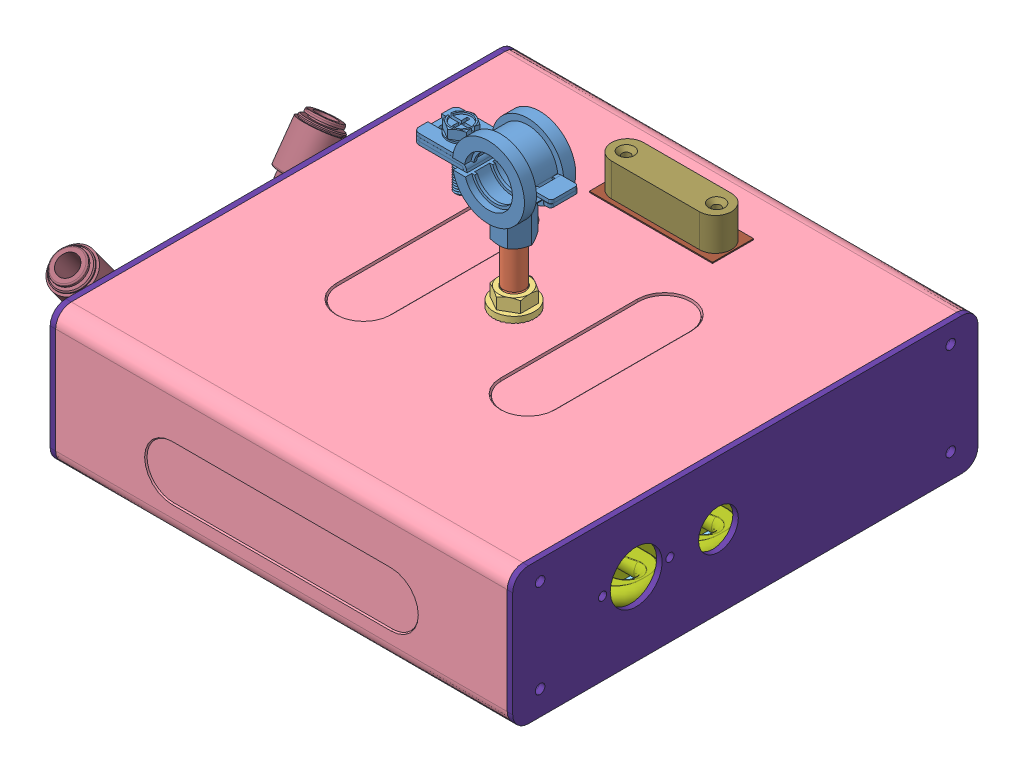
SolidWorks assembly LFR.101, configuration Default. Lengths in mm.
Overall size (264.18 207.36 215.9).
37 component instances, 17 part files, 64 mates.
Components (placement in the parent):
- 2615T130_VIBRATION-DAMPING CLAMPING HANGER-1: 2615T130_VIBRATION-DAMPING CLAMPING HANGER [2615T13] x (-1 0 0) z (0 0 1) size (60.33 44.72 23.81)
- 92386A632_SS THRD-LOCKING ADJUSTING   POSITIONING STUD-1: 92386A632_SS THRD-LOCKING ADJUSTING   POSITIONING STUD [92386A632] at (0 -65.8495 0) x (1 0 0) z (0 -1 0) size (10.08 10.01 51.87)
- 93776A461_TYPE 18-8 SS SERRATED-FLANGE LOCKNUT-1: 93776A461_TYPE 18-8 SS SERRATED-FLANGE LOCKNUT [93776A461] at (0 -47.3075 0) x (1 0 0) z (0 1 0) size (19.05 19.05 9.51)
- LFR.001-1: LFR.001 [BENT] at (0 -56.0388 0) size (209.55 64.1 215.9)
- LightPanel-1: LightPanel [Default] at (5.3651 -116.5988 -8.8508) x (0 0 -1) z (-1 0 0) size (195.78 12.57 210.82)
  - LightPCB-1: LightPCB [Default] at (-97.8524 -1.8098 101.8851) size (195.78 1.57 210.82)
  - KNAC36xxADS_Optic-1: KNAC36xxADS_Optic [Default] at (-8.8508 2.765 90.5129) x (0 0 1) z (0 1 0) size (193.04 178 11)
- aavid_heatsink-1: aavid_heatsink [Default] at (0.2 -114.7889 0) x (-1 0 0) z (0 0 -1) size (237.85 17.03 177.8)
- 92949A133_18-8 SS BUTTON-HEAD SOCKET CAP SCREW-1: 92949A133_18-8 SS BUTTON-HEAD SOCKET CAP SCREW [92949A133] at (100.965 -121.2151 93.4466) x (-0.331806 0 0.943348) z (0 -1 0) size (6.05 6.05 11.55)
- 94241A230_TYPE 316 STAINLESS STEEL SPLIT LOCK WASHER-1: 94241A230_TYPE 316 STAINLESS STEEL SPLIT LOCK WASHER [94241A230] at (100.965 -114.0269 93.4466) x (0.331806 0 -0.943348) z (0 -1 0) size (5.13 5.14 1.64)
- 90730A006_TYPE 18-8 STAINLESS STEEL NARROW HEX NUT-1: 90730A006_TYPE 18-8 STAINLESS STEEL NARROW HEX NUT [90730A006] at (100.965 -111.9978 93.4466) x (0.975805 0 0.218641) z (-0.218641 0 0.975805) size (6.35 2.87 7.33)
- 92949A133_18-8 SS BUTTON-HEAD SOCKET CAP SCREW-4: 92949A133_18-8 SS BUTTON-HEAD SOCKET CAP SCREW [92949A133] at (-100.965 -121.2151 93.4466) x (-0.331806 0 0.943348) z (0 -1 0) size (6.05 6.05 11.55)
- 92949A133_18-8 SS BUTTON-HEAD SOCKET CAP SCREW-5: 92949A133_18-8 SS BUTTON-HEAD SOCKET CAP SCREW [92949A133] at (100.965 -121.2151 -94.0054) x (-0.331806 0 0.943348) z (0 -1 0) size (6.05 6.05 11.55)
- 92949A133_18-8 SS BUTTON-HEAD SOCKET CAP SCREW-8: 92949A133_18-8 SS BUTTON-HEAD SOCKET CAP SCREW [92949A133] at (-100.965 -121.2151 -94.0054) x (-0.331806 0 0.943348) z (0 -1 0) size (6.05 6.05 11.55)
- 90730A006_TYPE 18-8 STAINLESS STEEL NARROW HEX NUT-4: 90730A006_TYPE 18-8 STAINLESS STEEL NARROW HEX NUT [90730A006] at (-100.965 -111.9978 93.4466) x (0.975805 0 0.218641) z (-0.218641 0 0.975805) size (6.35 2.87 7.33)
- 90730A006_TYPE 18-8 STAINLESS STEEL NARROW HEX NUT-5: 90730A006_TYPE 18-8 STAINLESS STEEL NARROW HEX NUT [90730A006] at (100.965 -111.9978 -94.0054) x (0.975805 0 0.218641) z (-0.218641 0 0.975805) size (6.35 2.87 7.33)
- 90730A006_TYPE 18-8 STAINLESS STEEL NARROW HEX NUT-8: 90730A006_TYPE 18-8 STAINLESS STEEL NARROW HEX NUT [90730A006] at (-100.965 -111.9978 -94.0054) x (0.975805 0 0.218641) z (-0.218641 0 0.975805) size (6.35 2.87 7.33)
- 94241A230_TYPE 316 STAINLESS STEEL SPLIT LOCK WASHER-4: 94241A230_TYPE 316 STAINLESS STEEL SPLIT LOCK WASHER [94241A230] at (-100.965 -114.0269 93.4466) x (0.331806 0 -0.943348) z (0 -1 0) size (5.13 5.14 1.64)
- 94241A230_TYPE 316 STAINLESS STEEL SPLIT LOCK WASHER-5: 94241A230_TYPE 316 STAINLESS STEEL SPLIT LOCK WASHER [94241A230] at (100.965 -114.0269 -94.0054) x (0.331806 0 -0.943348) z (0 -1 0) size (5.13 5.14 1.64)
- 94241A230_TYPE 316 STAINLESS STEEL SPLIT LOCK WASHER-8: 94241A230_TYPE 316 STAINLESS STEEL SPLIT LOCK WASHER [94241A230] at (-100.965 -114.0269 -94.0054) x (0.331806 0 -0.943348) z (0 -1 0) size (5.13 5.14 1.64)
- 76665A68_VHB_TAPE-1: 76665A68_VHB_TAPE [Default] at (0 -56.0388 -73.025) x (0 0 1) z (-1 0 0) size (19.05 0.51 57.15)
- 3338A22_HORIZONTAL_SURFACE_MOUNT_LEVEL-1: 3338A22_HORIZONTAL_SURFACE_MOUNT_LEVEL [Default] at (0.0625 -55.5307 -72.9641) size (55.63 15.24 14.83)
- 9406T170_PUSH-TO-CONNECT TUBE FITTING FOR SS TUBING-1: 9406T170_PUSH-TO-CONNECT TUBE FITTING FOR SS TUBING [9406T17] at (-147.214 -103.439 -45.2) x (0 -0.582087 -0.813127) z (1 0 0) size (19.3 35.05 39.88)
- 9406T170_PUSH-TO-CONNECT TUBE FITTING FOR SS TUBING-2: 9406T170_PUSH-TO-CONNECT TUBE FITTING FOR SS TUBING [9406T17] at (-147.214 -103.439 45) x (0 0.587828 -0.808986) z (1 0 0) size (19.3 35.05 39.88)
- 94639A303_NYLON UNTHREADED SPACERS-1: 94639A303_NYLON UNTHREADED SPACERS [94639A303] at (-40.44 -94.4389 -55.499) x (0.961212 0 0.275811) z (0 1 0) size (6.35 6.35 12.7)
- 94639A303_NYLON UNTHREADED SPACERS-2: 94639A303_NYLON UNTHREADED SPACERS [94639A303] at (40.84 -94.4389 -55.499) x (0.961212 0 0.275811) z (0 1 0) size (6.35 6.35 12.7)
- 94639A303_NYLON UNTHREADED SPACERS-3: 94639A303_NYLON UNTHREADED SPACERS [94639A303] at (40.84 -94.4389 55.499) x (0.961212 0 0.275811) z (0 1 0) size (6.35 6.35 12.7)
- 94639A303_NYLON UNTHREADED SPACERS-4: 94639A303_NYLON UNTHREADED SPACERS [94639A303] at (-40.44 -94.4389 55.499) x (0.961212 0 0.275811) z (0 1 0) size (6.35 6.35 12.7)
- 92949A151_18-8 SS BUTTON-HEAD SOCKET CAP SCREW-1: 92949A151_18-8 SS BUTTON-HEAD SOCKET CAP SCREW [92949A151] at (-40.44 -84.4567 -55.499) x (0.994916 0 -0.100706) z (0 1 0) size (6.65 6.65 21.35)
- 92949A151_18-8 SS BUTTON-HEAD SOCKET CAP SCREW-2: 92949A151_18-8 SS BUTTON-HEAD SOCKET CAP SCREW [92949A151] at (-40.44 -84.4567 55.499) x (0.991359 0 -0.131179) z (0 1 0) size (6.65 6.65 21.35)
- 92949A151_18-8 SS BUTTON-HEAD SOCKET CAP SCREW-3: 92949A151_18-8 SS BUTTON-HEAD SOCKET CAP SCREW [92949A151] at (40.84 -84.4567 55.499) x (0.991359 0 -0.131179) z (0 1 0) size (6.65 6.65 21.35)
- 92949A151_18-8 SS BUTTON-HEAD SOCKET CAP SCREW-4: 92949A151_18-8 SS BUTTON-HEAD SOCKET CAP SCREW [92949A151] at (40.84 -84.4567 -55.499) x (0.991359 0 -0.131179) z (0 1 0) size (6.65 6.65 21.35)
- light_controller v16-1: light_controller v16 [Default] at (-45.52 -88.0889 -60.579) x (0 0 1) z (0 1 0) size (121.16 91.44 17.03)
- LFR.008-1: LFR.008 [Front-1] at (-102.235 -158.9087 0) x (0 0 1) z (-1 0 0) size (215.9 131.44 2.54)
- LFR.008-2: LFR.008 [Front-2] at (-104.775 -87.7887 0) x (0 0 1) z (-1 0 0) size (215.9 131.44 2.54)
- LFR.008-3: LFR.008 [Back1] at (104.775 -158.9087 0) x (0 0 1) z (-1 0 0) size (215.9 131.44 2.54)
- LFR.008-4: LFR.008 [Back2] at (107.315 -87.7887 0) x (0 0 1) z (-1 0 0) size (215.9 131.44 2.54)
Mates (geometry in assembly coordinates):
- Coincident1: coincident: plane of 2615T130_VIBRATION-DAMPING CLAMPING HANGER-1 through (0 0 0) normal (0 0 1); plane of assembly through (0 0 0) normal (0 0 1)
- Coincident2: coincident: plane of 2615T130_VIBRATION-DAMPING CLAMPING HANGER-1 through (0 0 0) normal (0 -1 0); plane of assembly through (0 0 0) normal (0 1 0)
- Coincident3: coincident: plane of 2615T130_VIBRATION-DAMPING CLAMPING HANGER-1 through (0 0 0) normal (-1 0 0); plane of assembly through (0 0 0) normal (1 0 0)
- Concentric1: concentric: cylinder of 2615T130_VIBRATION-DAMPING CLAMPING HANGER-1 through (0 16.7015 0) axis (0 -1 0) radius 5.3975; cylinder of 92386A632_SS THRD-LOCKING ADJUSTING   POSITIONING STUD-1 through (0 -15.0495 0) axis (0 1 0) radius 4.7625
- Coincident4: coincident: plane of 2615T130_VIBRATION-DAMPING CLAMPING HANGER-1 through (-8.1389 -27.7495 0) normal (0 -1 0); plane of 92386A632_SS THRD-LOCKING ADJUSTING   POSITIONING STUD-1 through (0 -27.7495 0) normal (0 1 0)
- Concentric2: concentric: cylinder of LFR.001-1 through (0 -59.2138 0) axis (0 -1 0) radius 7.112; cylinder of 92386A632_SS THRD-LOCKING ADJUSTING   POSITIONING STUD-1 through (0 -15.0495 0) axis (0 1 0) radius 4.7625
- Concentric3: concentric: cylinder of 93776A461_TYPE 18-8 SS SERRATED-FLANGE LOCKNUT-1 through (0 -53.0669 0) axis (0 -1 0) radius 9.525; cylinder of 92386A632_SS THRD-LOCKING ADJUSTING   POSITIONING STUD-1 through (0 -15.0495 0) axis (0 1 0) radius 4.7625
- Coincident5: coincident: plane of LFR.001-1 through (-104.775 -56.0388 107.95) normal (0 1 0); point of 93776A461_TYPE 18-8 SS SERRATED-FLANGE LOCKNUT-1
- Parallel1: parallel: plane of 2615T130_VIBRATION-DAMPING CLAMPING HANGER-1 through (-36.83 -3.1877 33.5953) normal (-1 0 0); plane of LFR.001-1 through (-104.775 -59.2138 107.95) normal (-1 0 0)
- Distance1: distance = 0.508 mm: plane of 93776A461_TYPE 18-8 SS SERRATED-FLANGE LOCKNUT-1 through (-7.1437 -47.3075 -12.3733) normal (0 1 0); plane of 92386A632_SS THRD-LOCKING ADJUSTING   POSITIONING STUD-1 through (0 -46.7995 0) normal (0 -1 0)
- Coincident6: coincident: plane of LightPanel-1/LightPCB-1 through (-96.52 -114.7889 89.0016) normal (0 1 0); plane of aavid_heatsink-1 through (0.2 -114.7889 0) normal (0 -1 0)
- Distance2: distance = 29.21 mm: plane of aavid_heatsink-1 through (76.2 -100.7889 88.9) normal (1 0 0); plane of LightPanel-1/LightPCB-1 through (105.41 -116.3637 -97.8916) normal (1 0 0)
- Coincident8: coincident: plane of LFR.001-1 through (0 -116.3637 0) normal (0 1 0); plane of LightPanel-1/LightPCB-1 through (-96.52 -116.3637 89.0016) normal (0 -1 0)
- Width3: width: plane of aavid_heatsink-1 through (76.2 -100.7889 -88.9) normal (0 0 -1); plane of aavid_heatsink-1 through (76.2 -100.7889 88.9) normal (0 0 1); plane of LightPanel-1/LightPCB-1 through (105.41 -116.3637 97.8916) normal (0 0 1); plane of LightPanel-1/LightPCB-1 through (-105.41 -116.3637 -97.8916) normal (0 0 -1)
- Parallel2: parallel: plane of LFR.001-1 through (104.775 -56.0388 107.95) normal (1 0 0); plane of aavid_heatsink-1 through (76.2 -100.7889 88.9) normal (1 0 0)
- Width4: width: plane of LFR.001-1 through (0 -56.0388 107.95) normal (0 0 1); plane of LFR.001-1 through (0 -56.0388 -107.95) normal (0 0 -1); plane of aavid_heatsink-1 through (76.2 -100.7889 -88.9) normal (0 0 -1); plane of aavid_heatsink-1 through (76.2 -100.7889 88.9) normal (0 0 1)
- Width5: width: plane of LightPanel-1/LightPCB-1 through (105.41 -116.3637 -97.8916) normal (1 0 0); plane of LightPanel-1/LightPCB-1 through (-105.41 -116.3637 97.8916) normal (-1 0 0); plane of LFR.001-1 through (104.775 -59.2138 107.95) normal (1 0 0); plane of LFR.001-1 through (-104.775 -119.5387 107.95) normal (-1 0 0)
- Concentric4: concentric: cylinder of LightPanel-1/LightPCB-1 through (100.965 -116.3637 93.4466) axis (0 1 0) radius 1.778; cylinder of 92949A133_18-8 SS BUTTON-HEAD SOCKET CAP SCREW-1 through (100.965 -121.2151 93.4466) axis (0 -1 0) radius 3.0226
- Coincident11: coincident: plane of LightPanel-1/LightPCB-1 through (-96.52 -114.7889 89.0016) normal (0 1 0); point of 94241A230_TYPE 316 STAINLESS STEEL SPLIT LOCK WASHER-1
- Parallel3: parallel: plane of LightPanel-1/LightPCB-1 through (-96.52 -114.7889 89.0016) normal (0 1 0); plane of 94241A230_TYPE 316 STAINLESS STEEL SPLIT LOCK WASHER-1 through (100.965 -114.0269 93.4466) normal (0 -1 0)
- Coincident13: coincident: plane of 92949A133_18-8 SS BUTTON-HEAD SOCKET CAP SCREW-1 through (100.965 -121.2151 93.4466) normal (-0.331806 0 0.943348); plane of 94241A230_TYPE 316 STAINLESS STEEL SPLIT LOCK WASHER-1 through (100.965 -114.0269 93.4466) normal (0.331806 0 -0.943348)
- Coincident14: coincident: plane of 92949A133_18-8 SS BUTTON-HEAD SOCKET CAP SCREW-1 through (100.965 -121.2151 93.4466) normal (-0.943348 0 -0.331806); plane of 94241A230_TYPE 316 STAINLESS STEEL SPLIT LOCK WASHER-1 through (100.965 -114.0269 93.4466) normal (0.943348 0 0.331806)
- Coincident15: coincident: plane of LFR.001-1 through (0 -119.5387 0) normal (0 -1 0); plane of 92949A133_18-8 SS BUTTON-HEAD SOCKET CAP SCREW-1 through (103.8164 -119.5387 94.4495) normal (0 1 0)
- Concentric5: concentric: cylinder of 92949A133_18-8 SS BUTTON-HEAD SOCKET CAP SCREW-1 through (100.965 -121.2151 93.4466) axis (0 -1 0) radius 3.0226; circle of 90730A006_TYPE 18-8 STAINLESS STEEL NARROW HEX NUT-1
- Coincident16: coincident: point of 94241A230_TYPE 316 STAINLESS STEEL SPLIT LOCK WASHER-1; plane of 90730A006_TYPE 18-8 STAINLESS STEEL NARROW HEX NUT-1 through (98.2676 -113.1884 90.9637) normal (0 -1 0)
- Coincident17: coincident: plane of LFR.001-1 through (-104.775 -56.0388 107.95) normal (0 1 0); plane of 76665A68_VHB_TAPE-1 through (0 -56.0388 -73.025) normal (0 -1 0)
- Distance3: distance = 25.4 mm: plane of 76665A68_VHB_TAPE-1 through (28.575 -55.5307 -82.55) normal (0 0 -1); plane of LFR.001-1 through (0 -56.0388 -107.95) normal (0 0 -1)
- Width6: width: plane of 76665A68_VHB_TAPE-1 through (-28.575 -55.5307 -82.55) normal (-1 0 0); plane of 76665A68_VHB_TAPE-1 through (28.575 -55.5307 -82.55) normal (1 0 0); plane of LFR.001-1 through (104.775 -56.0388 107.95) normal (1 0 0); plane of LFR.001-1 through (-104.775 -59.2138 107.95) normal (-1 0 0)
- Coincident19: coincident: plane of 76665A68_VHB_TAPE-1 through (0 -55.5307 -73.025) normal (0 1 0); plane of 3338A22_HORIZONTAL_SURFACE_MOUNT_LEVEL-1 through (-20.3337 -55.5307 -72.9641) normal (0 -1 0)
- Concentric6: concentric: cylinder of aavid_heatsink-1 through (87.28 -103.439 -45.2) axis (-1 0 0) radius 4.75; cylinder of 9406T170_PUSH-TO-CONNECT TUBE FITTING FOR SS TUBING-1 through (-116.988 -103.439 -45.2) axis (1 0 0) radius 4.7625
- Coincident20: coincident: plane of aavid_heatsink-1 through (-136.8 -103.439 -45.2) normal (-1 0 0); plane of 9406T170_PUSH-TO-CONNECT TUBE FITTING FOR SS TUBING-1 through (-136.8 -99.5664 -47.9722) normal (1 0 0)
- Coincident21: coincident: plane of 9406T170_PUSH-TO-CONNECT TUBE FITTING FOR SS TUBING-1 through (-139.2765 -97.1138 -49.7279) normal (-1 0 0); plane of 9406T170_PUSH-TO-CONNECT TUBE FITTING FOR SS TUBING-2 through (-139.2765 -97.146 49.5726) normal (-1 0 0)
- Concentric7: concentric: cylinder of aavid_heatsink-1 through (87.28 -103.439 45) axis (-1 0 0) radius 4.75; cylinder of 9406T170_PUSH-TO-CONNECT TUBE FITTING FOR SS TUBING-2 through (-116.988 -103.439 45) axis (1 0 0) radius 9.652
- Concentric8: concentric: cylinder of aavid_heatsink-1 through (-40.44 -113.489 -55.499) axis (0 1 0) radius 1.3526; cylinder of 94639A303_NYLON UNTHREADED SPACERS-1 through (-40.44 -88.0889 -55.499) axis (0 -1 0) radius 3.175
- Coincident22: coincident: plane of aavid_heatsink-1 through (0.2 -100.7889 0) normal (0 1 0); plane of 94639A303_NYLON UNTHREADED SPACERS-1 through (-40.44 -100.7889 -55.499) normal (0 -1 0)
- Coincident23: coincident: plane of 94639A303_NYLON UNTHREADED SPACERS-1 through (-40.44 -88.0889 -55.499) normal (0 1 0); plane of 94639A303_NYLON UNTHREADED SPACERS-4 through (-40.44 -88.0889 55.499) normal (0 1 0)
- Coincident24: coincident: plane of 94639A303_NYLON UNTHREADED SPACERS-2 through (40.84 -88.0889 -55.499) normal (0 1 0); plane of 94639A303_NYLON UNTHREADED SPACERS-3 through (40.84 -88.0889 55.499) normal (0 1 0)
- Coincident25: coincident: plane of 94639A303_NYLON UNTHREADED SPACERS-3 through (40.84 -88.0889 55.499) normal (0 1 0); plane of 94639A303_NYLON UNTHREADED SPACERS-4 through (-40.44 -88.0889 55.499) normal (0 1 0)
- Concentric9: concentric: cylinder of aavid_heatsink-1 through (40.84 -113.489 -55.499) axis (0 1 0) radius 1.3526; cylinder of 94639A303_NYLON UNTHREADED SPACERS-2 through (40.84 -88.0889 -55.499) axis (0 -1 0) radius 3.175
- Concentric10: concentric: cylinder of aavid_heatsink-1 through (-40.44 -113.489 55.499) axis (0 1 0) radius 1.3526; cylinder of 94639A303_NYLON UNTHREADED SPACERS-4 through (-40.44 -88.0889 55.499) axis (0 -1 0) radius 3.175
- Concentric11: concentric: cylinder of aavid_heatsink-1 through (40.84 -113.489 55.499) axis (0 1 0) radius 1.3526; cylinder of 94639A303_NYLON UNTHREADED SPACERS-3 through (40.84 -88.0889 55.499) axis (0 -1 0) radius 3.175
- Concentric12: concentric: cylinder of 94639A303_NYLON UNTHREADED SPACERS-1 through (-40.44 -88.0889 -55.499) axis (0 -1 0) radius 3.175; cylinder of 92949A151_18-8 SS BUTTON-HEAD SOCKET CAP SCREW-1 through (-40.44 -84.4567 -55.499) axis (0 1 0) radius 3.3274
- Coincident26: coincident: plane of 92949A151_18-8 SS BUTTON-HEAD SOCKET CAP SCREW-1 through (-40.1049 -86.3109 -52.1885) normal (0 -1 0); plane of 92949A151_18-8 SS BUTTON-HEAD SOCKET CAP SCREW-3 through (41.2765 -86.3109 58.7976) normal (0 -1 0)
- Coincident27: coincident: plane of 92949A151_18-8 SS BUTTON-HEAD SOCKET CAP SCREW-3 through (41.2765 -86.3109 58.7976) normal (0 -1 0); plane of 92949A151_18-8 SS BUTTON-HEAD SOCKET CAP SCREW-4 through (41.2765 -86.3109 -52.2004) normal (0 -1 0)
- Coincident28: coincident: plane of 92949A151_18-8 SS BUTTON-HEAD SOCKET CAP SCREW-2 through (-40.0035 -86.3109 58.7976) normal (0 -1 0); plane of 92949A151_18-8 SS BUTTON-HEAD SOCKET CAP SCREW-4 through (41.2765 -86.3109 -52.2004) normal (0 -1 0)
- Concentric13: concentric: cylinder of 94639A303_NYLON UNTHREADED SPACERS-3 through (40.84 -88.0889 55.499) axis (0 -1 0) radius 3.175; cylinder of 92949A151_18-8 SS BUTTON-HEAD SOCKET CAP SCREW-3 through (40.84 -84.4567 55.499) axis (0 1 0) radius 3.3274
- Concentric14: concentric: cylinder of 94639A303_NYLON UNTHREADED SPACERS-2 through (40.84 -88.0889 -55.499) axis (0 -1 0) radius 3.175; cylinder of 92949A151_18-8 SS BUTTON-HEAD SOCKET CAP SCREW-4 through (40.84 -84.4567 -55.499) axis (0 1 0) radius 3.3274
- Concentric15: concentric: cylinder of 94639A303_NYLON UNTHREADED SPACERS-4 through (-40.44 -88.0889 55.499) axis (0 -1 0) radius 3.175; cylinder of 92949A151_18-8 SS BUTTON-HEAD SOCKET CAP SCREW-2 through (-40.44 -84.4567 55.499) axis (0 1 0) radius 3.3274
- Distance4: distance = 1.778 mm: plane of 92949A151_18-8 SS BUTTON-HEAD SOCKET CAP SCREW-1 through (-40.1049 -86.3109 -52.1885) normal (0 -1 0); plane of 94639A303_NYLON UNTHREADED SPACERS-1 through (-40.44 -88.0889 -55.499) normal (0 1 0)
- Concentric19: concentric: cylinder of 94639A303_NYLON UNTHREADED SPACERS-1 through (-40.44 -88.0889 -55.499) axis (0 -1 0) radius 3.175; cylinder of light_controller v16-1 through (-40.44 -88.0889 -55.499) axis (0 1 0) radius 1.905
- Parallel7: parallel: plane of aavid_heatsink-1 through (76.2 -100.7889 -88.9) normal (0 0 -1); plane of light_controller v16-1 through (45.92 -88.0889 -60.579) normal (0 0 -1)
- Coincident30: coincident: plane of 94639A303_NYLON UNTHREADED SPACERS-1 through (-40.44 -88.0889 -55.499) normal (0 1 0); plane of light_controller v16-1 through (0.2 -88.0889 0) normal (0 -1 0)
- Concentric20: concentric: cylinder of LFR.008-1 through (-104.775 -103.439 -45.2) axis (1 0 0) radius 5.08; cylinder of LFR.008-2 through (-107.315 -103.439 -45.2) axis (1 0 0) radius 5.08
- Coincident31: coincident: plane of LFR.008-1 through (-104.775 -63.2777 100.711) normal (-1 0 0); plane of LFR.008-2 through (-104.775 -63.2777 -100.711) normal (1 0 0)
- Coincident32: coincident: plane of LFR.001-1 through (-104.775 -59.2138 -107.95) normal (-1 0 0); plane of LFR.008-2 through (-104.775 -63.2777 -100.711) normal (1 0 0)
- Concentric21: concentric: cylinder of aavid_heatsink-1 through (87.28 -103.439 45) axis (-1 0 0) radius 4.75; cylinder of LFR.008-2 through (-107.315 -103.439 45) axis (1 0 0) radius 5.08
- Concentric22: concentric: cylinder of aavid_heatsink-1 through (87.28 -103.439 45) axis (-1 0 0) radius 4.75; cylinder of LFR.008-1 through (-104.775 -103.439 45) axis (1 0 0) radius 5.08
- Concentric23: concentric: cylinder of aavid_heatsink-1 through (87.28 -103.439 -45.2) axis (-1 0 0) radius 4.75; cylinder of LFR.008-2 through (-107.315 -103.439 -45.2) axis (1 0 0) radius 5.08
- Coincident34: coincident: plane of LFR.008-2 through (-107.315 -63.2777 -107.95) normal (0 0 -1); plane of LFR.008-4 through (104.775 -63.2777 -107.95) normal (0 0 -1)
- Coincident35: coincident: plane of LFR.008-2 through (-107.315 -119.5387 52.4295) normal (0 -1 0); plane of LFR.008-4 through (104.775 -119.5387 52.4295) normal (0 -1 0)
- Coincident37: coincident: plane of LFR.008-3 through (104.775 -63.2777 100.711) normal (1 0 0); plane of LFR.008-4 through (104.775 -63.2777 -100.711) normal (-1 0 0)
- Width8: width: plane of LFR.008-4 through (104.775 -112.2998 107.95) normal (0 0 1); plane of LFR.008-4 through (104.775 -63.2777 -107.95) normal (0 0 -1); plane of LFR.008-3 through (102.235 -63.2777 -104.775) normal (0 0 -1); plane of LFR.008-3 through (102.235 -108.5637 104.775) normal (0 0 1)
- Coincident40: coincident: plane of LFR.001-1 through (-104.775 -59.2138 107.95) normal (0 -1 0); plane of LFR.008-3 through (102.235 -59.2138 100.711) normal (0 1 0)
- Coincident41: coincident: plane of LFR.001-1 through (104.775 -119.5387 104.775) normal (1 0 0); plane of LFR.008-4 through (104.775 -63.2777 -100.711) normal (-1 0 0)
